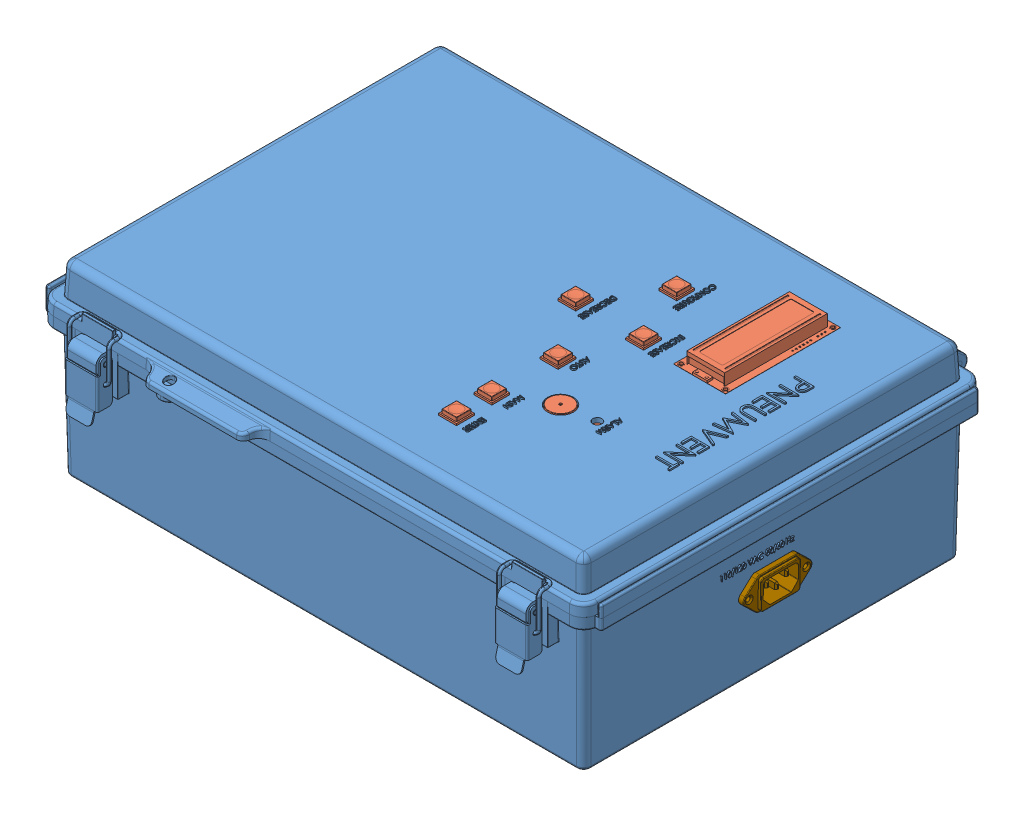
SolidWorks assembly Assem1, configuration Default. Lengths in mm.
Overall size (388.4 140.28 306.16).
18 component instances, 11 part files, 28 mates.
Components (placement in the parent):
- WQ-64-1: WQ-64 [Default] at (79.8342 238.8008 332.3502) size (388.4 133 306.16)
- Pneumvent_PCB-2: Pneumvent_PCB [Default] at (25.1243 261.9317 460.891) x (0 0 -1) z (0 -1 0) size (211.94 152.65 31.54)
- 2-2-Air-Selonoid-Valve-1: 2-2-Air-Selonoid-Valve [Default] at (115.9625 193.5208 210.1421) x (-0.999997 0.002311 -0.00004) z (0 -0.017452 -0.999848) size (31 21.15 9.8)
- 2-2-Electrovalve-plates-1: 2-2-Electrovalve-plates [Default] at (96.4894 183.5228 207.7662) x (-0.999997 0.002311 -0.00004) z (0 -0.017452 -0.999848) size (19.3 10 14.9)
- 2-2-Electrovalve-plates-2: 2-2-Electrovalve-plates [Default] at (59.8025 183.0258 207.7749) x (1 0 0) z (0 0.017452 0.999848) size (19.3 10 14.9)
- 2-2-Air-Selonoid-Valve-2: 2-2-Air-Selonoid-Valve [Default] at (40.3525 192.9798 205.0507) x (1 0 0) z (0 0.017452 0.999848) size (31 21.15 9.8)
- 3-2-Air-Selonoid-Valve-1: 3-2-Air-Selonoid-Valve [Default] at (191.2838 194.7411 210.1208) x (-1 0 0) z (0 -0.017452 -0.999848) size (31 21.15 9.8)
- 3-2-Electr0valve-plates-1: 3-2-Electr0valve-plates [Default] at (171.8338 184.6982 207.7457) x (-1 0 0) z (0 -0.017452 -0.999848) size (19.3 10 14.9)
- 3-2-Electr0valve-plates-2: 3-2-Electr0valve-plates [Default] at (132.6376 184.1841 207.7547) x (-1 0 0) z (0 -0.017452 -0.999848) size (19.3 10 14.9)
- 3-2-Air-Selonoid-Valve-2: 3-2-Air-Selonoid-Valve [Default] at (152.0876 194.2271 210.1297) x (-1 0 0) z (0 -0.017452 -0.999848) size (31 21.15 9.8)
- Fitting-1: Fitting [Default] at (177.2838 189.0675 200.2183) x (-1 0 0) z (0 -0.017452 -0.999848) size (8 9.8 15.7)
- Fitting-2: Fitting [Default] at (138.0876 188.5534 200.2272) x (-1 0 0) z (0 -0.017452 -0.999848) size (8 9.8 15.7)
- Fitting-3: Fitting [Default] at (54.3525 187.6551 215.1452) x (1 0 0) z (0 0.017452 0.999848) size (8 9.8 15.7)
- Fitting-4: Fitting [Default] at (101.9498 187.8794 200.239) x (0.141326 -0.989812 0.017277) z (0 -0.017452 -0.999848) size (8 9.8 15.7)
- Fuente meanwell LRS-200-12-1: Fuente meanwell LRS-200-12 [Default] at (108.9557 139.9374 59.9923) x (-1 0 0) z (0 1 0) size (215 115.05 30.05) (hidden)
- User Library-Schaffner_FN9222R-1-06_filtered_IEC_inlet.step-2: User Library-Schaffner_FN9222R-1-06_filtered_IEC_inlet.step [Default] at (262.0482 193.77 332.4054) x (0 0 -1) z (-0.999848 0.017452 0) size (48 22.5 57.5)
- Continental Hydraulics-VED03M-3 K1 SOL DES C.step-1: Continental Hydraulics-VED03M-3 K1 SOL DES C.step [Default] at (100.1559 162.8008 404.1936) size (207 88.89 46)
- Battery-1: Battery [Default] at (-72.9724 138.8008 412.0423) x (0 0 -1) z (1 0 0) size (150.67 100.33 50.29)
Mates (geometry in assembly coordinates):
- Concentric2: concentric anti-aligned: cylinder of 2-2-Air-Selonoid-Valve-1 through (93.4559 190.6165 206.9423) axis (0.002311 0.999845 -0.017452) radius 0.8; cylinder of 2-2-Electrovalve-plates-1 through (93.4626 193.516 206.8917) axis (-0.002311 -0.999845 0.017452) radius 0.6105
- Concentric3: concentric anti-aligned: cylinder of 2-2-Electrovalve-plates-2 through (62.8525 193.0365 208.3002) axis (0 -0.999848 0.017452) radius 0.6105; cylinder of 2-2-Air-Selonoid-Valve-2 through (62.8525 190.1369 208.3508) axis (0 0.999848 -0.017452) radius 0.8
- Concentric4: concentric anti-aligned: cylinder of 3-2-Air-Selonoid-Valve-1 through (168.7838 191.7849 206.9219) axis (0 0.999848 -0.017452) radius 0.8; cylinder of 3-2-Electr0valve-plates-1 through (168.7838 194.6844 206.8713) axis (0 -0.999848 0.017452) radius 0.6105
- Concentric5: concentric anti-aligned: cylinder of 3-2-Electr0valve-plates-2 through (129.5876 194.1703 206.8802) axis (0 -0.999848 0.017452) radius 0.6105; cylinder of 3-2-Air-Selonoid-Valve-2 through (129.5876 191.2708 206.9308) axis (0 0.999848 -0.017452) radius 0.8
- Concentric6: concentric aligned: circle of 3-2-Electr0valve-plates-1; cylinder of Fitting-1 through (177.2838 189.1111 202.7179) axis (0 -0.017452 -0.999848) radius 1.5
- Concentric9: concentric aligned: cylinder of 2-2-Electrovalve-plates-1 through (101.9498 187.8794 200.239) axis (0 -0.017452 -0.999848) radius 1.2295; cylinder of Fitting-4 through (101.9498 187.9231 202.7386) axis (0 -0.017452 -0.999848) radius 1.5
- Concentric10: concentric aligned: cylinder of 2-2-Electrovalve-plates-2 through (54.3525 187.6551 215.1452) axis (0 0.017452 0.999848) radius 1.2295; cylinder of Fitting-3 through (54.3525 187.6115 212.6456) axis (0 0.017452 0.999848) radius 1.5
- Concentric11: concentric aligned: cylinder of 3-2-Electr0valve-plates-2 through (138.0876 188.5534 200.2272) axis (0 -0.017452 -0.999848) radius 1.2295; cylinder of Fitting-2 through (138.0876 188.597 202.7269) axis (0 -0.017452 -0.999848) radius 1.5
- Coincident1: coincident anti-aligned: plane of 2-2-Electrovalve-plates-1 through (105.6625 193.37 200.1432) normal (0 -0.017452 -0.999848); plane of Fitting-4 through (99.2274 187.4909 200.2458) normal (0 0.017452 0.999848)
- Coincident2: coincident anti-aligned: plane of 2-2-Air-Selonoid-Valve-1 through (86.9294 193.5076 205.5416) normal (-0.002311 -0.999845 0.017452); plane of 2-2-Electrovalve-plates-1 through (105.6625 193.3788 200.6431) normal (0.002311 0.999845 -0.017452)
- Coincident3: coincident anti-aligned: plane of 2-2-Electrovalve-plates-2 through (50.6525 193.1456 214.5493) normal (0 0.999848 -0.017452); plane of 2-2-Air-Selonoid-Valve-2 through (69.3857 193.0601 209.65) normal (0 -0.999848 0.017452)
- Coincident4: coincident anti-aligned: plane of 2-2-Electrovalve-plates-2 through (50.6525 193.1543 215.0492) normal (0 0.017452 0.999848); plane of Fitting-3 through (54.3525 190.4047 215.0972) normal (0 -0.017452 -0.999848)
- Coincident5: coincident aligned: plane of WQ-64-1 through (79.8342 138.8008 332.3502) normal (0 -1 0); plane of Continental Hydraulics-VED03M-3 K1 SOL DES C.step-1 through (132.6559 138.8008 427.1936) normal (0 -1 0)
- Coincident7: coincident anti-aligned: plane of WQ-64-1 through (262.8342 238.8008 465.3502) normal (0.999848 -0.017452 0); plane of User Library-Schaffner_FN9222R-1-06_filtered_IEC_inlet.step-2 through (261.9868 190.2494 312.4054) normal (-0.999848 0.017452 0)
- Coincident8: coincident anti-aligned: plane of 3-2-Electr0valve-plates-1 through (180.9838 194.5666 200.1223) normal (0 -0.017452 -0.999848); plane of Fitting-1 through (177.2838 191.817 200.1703) normal (0 0.017452 0.999848)
- Coincident9: coincident anti-aligned: plane of 3-2-Air-Selonoid-Valve-1 through (162.2506 194.6609 205.5215) normal (0 -0.999848 0.017452); plane of 3-2-Electr0valve-plates-1 through (180.9838 194.5754 200.6222) normal (0 0.999848 -0.017452)
- Coincident10: coincident anti-aligned: plane of 3-2-Electr0valve-plates-2 through (141.7876 194.0525 200.1313) normal (0 -0.017452 -0.999848); plane of Fitting-2 through (138.0876 191.303 200.1793) normal (0 0.017452 0.999848)
- Coincident11: coincident anti-aligned: plane of 3-2-Electr0valve-plates-2 through (141.7876 194.0613 200.6312) normal (0 0.999848 -0.017452); plane of 3-2-Air-Selonoid-Valve-2 through (123.0544 194.1468 205.5304) normal (0 -0.999848 0.017452)
- Coincident12: coincident aligned: plane of WQ-64-1 through (79.8342 138.8008 332.3502) normal (0 -1 0); plane of Battery-1 through (-22.6804 138.8008 412.0423) normal (0 -1 0)
- Concentric12: concentric aligned: cylinder of 2-2-Air-Selonoid-Valve-1 through (102.4625 193.552 210.1415) axis (0.002311 0.999845 -0.017452) radius 15; cylinder of 2-2-Electrovalve-plates-1 through (102.4556 190.5524 210.1939) axis (0.002311 0.999845 -0.017452) radius 15
- Parallel1: parallel anti-aligned: plane of WQ-64-1 through (262.8342 238.8008 199.3502) normal (0 -0.017452 -0.999848); plane of 2-2-Air-Selonoid-Valve-1 through (86.9634 208.3711 214.7836) normal (0 0.017452 0.999848)
- Concentric13: concentric anti-aligned: cylinder of 3-2-Air-Selonoid-Valve-1 through (177.7838 209.4389 209.8642) axis (0 -0.999848 0.017452) radius 16.5; cylinder of 3-2-Electr0valve-plates-1 through (177.7838 191.7416 210.1731) axis (0 0.999848 -0.017452) radius 15
- Concentric14: concentric anti-aligned: cylinder of 2-2-Electrovalve-plates-2 through (53.8525 189.9802 205.1031) axis (0 0.999848 -0.017452) radius 15; cylinder of 2-2-Air-Selonoid-Valve-2 through (53.8525 207.6775 204.7942) axis (0 -0.999848 0.017452) radius 16.5
- Concentric15: concentric anti-aligned: cylinder of 3-2-Electr0valve-plates-2 through (138.5876 191.2275 210.1821) axis (0 0.999848 -0.017452) radius 15; cylinder of 3-2-Air-Selonoid-Valve-2 through (138.5876 208.9248 209.8732) axis (0 -0.999848 0.017452) radius 16.5
- Coincident18: coincident aligned: plane of 2-2-Electrovalve-plates-2 through (68.9525 192.8943 200.1515) normal (0 -0.017452 -0.999848); plane of WQ-64-1 through (262.8342 238.8008 199.3502) normal (0 -0.017452 -0.999848)
- Coincident20: coincident aligned: plane of WQ-64-1 through (262.8342 238.8008 199.3502) normal (0 -0.017452 -0.999848); plane of 2-2-Electrovalve-plates-1 through (105.6625 193.37 200.1432) normal (0 -0.017452 -0.999848)
- Coincident26: coincident aligned: plane of WQ-64-1 through (262.8342 238.8008 199.3502) normal (0 -0.017452 -0.999848); plane of 3-2-Electr0valve-plates-1 through (180.9838 194.5666 200.1223) normal (0 -0.017452 -0.999848)
- Coincident27: coincident aligned: plane of WQ-64-1 through (262.8342 238.8008 199.3502) normal (0 -0.017452 -0.999848); plane of 3-2-Electr0valve-plates-2 through (141.7876 194.0525 200.1313) normal (0 -0.017452 -0.999848)
